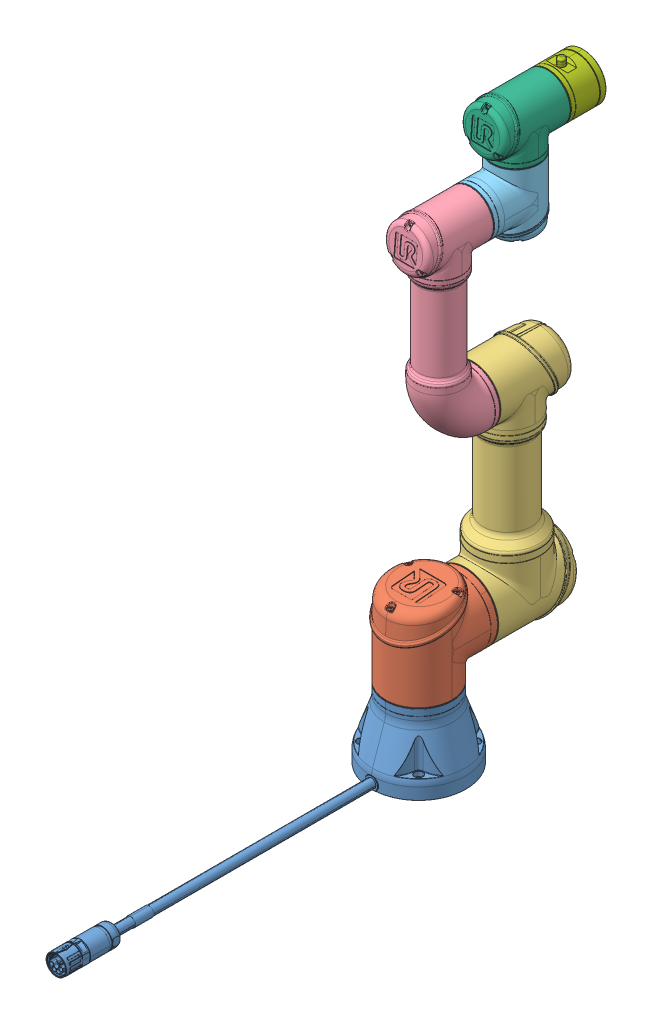
SolidWorks assembly eSeries_UR3e_B, configuration Default. Lengths in mm.
Overall size (128 755.25 714.57).
8 component instances, 7 part files, 0 mates.
Components (placement in the parent):
- eSeries_UR3e.STEP-1: eSeries_UR3e.STEP [Default] at origin size (128 755.25 714.57)
  - Copy of Base_UR3_G5^1000513.STEP-1: Copy of Base_UR3_G5^1000513.STEP [Default] at origin size (128 108.76 555.42)
  - Copy of Link1_UR3_G5^1000513.STEP-1: Copy of Link1_UR3_G5^1000513.STEP [Default] at (0 151.85 0) x (0 0 1) z (-1 0 0) size (172.26 115.55 106.56)
  - Copy of Link2_UR3_G5^1000513.STEP-1: Copy of Link2_UR3_G5^1000513.STEP [Default] at (0 151.85 -119.85) x (0 -1 0) z (1 0 0) size (341.2 115.55 105.37)
  - Copy of Link3_UR3_G5^1000513.STEP-1: Copy of Link3_UR3_G5^1000513.STEP [Default] at (0 608.6 -27) x (0 -1 0) z (-1 0 0) size (298.22 93.47 75.49)
  - Copy of Link4_UR3_G5^1000513.STEP-1: Copy of Link4_UR3_G5^1000513.STEP [Default] at (0 608.6 -131.05) x (0 0 1) z (1 0 0) size (93.87 90 69)
  - Copy of Link5_UR3_G5^1000513.STEP-1: Copy of Link5_UR3_G5^1000513.STEP [Default] at (0 693.95 -131.05) x (0 -1 0) z (-1 0 0) size (90.18 90.02 69)
  - Copy of Link6_UR3_G5^1000513.STEP-1: Copy of Link6_UR3_G5^1000513.STEP [Default] at (0 693.95 -223.15) x (-1 0 0) z (0 0 1) size (63 69.35 49)
